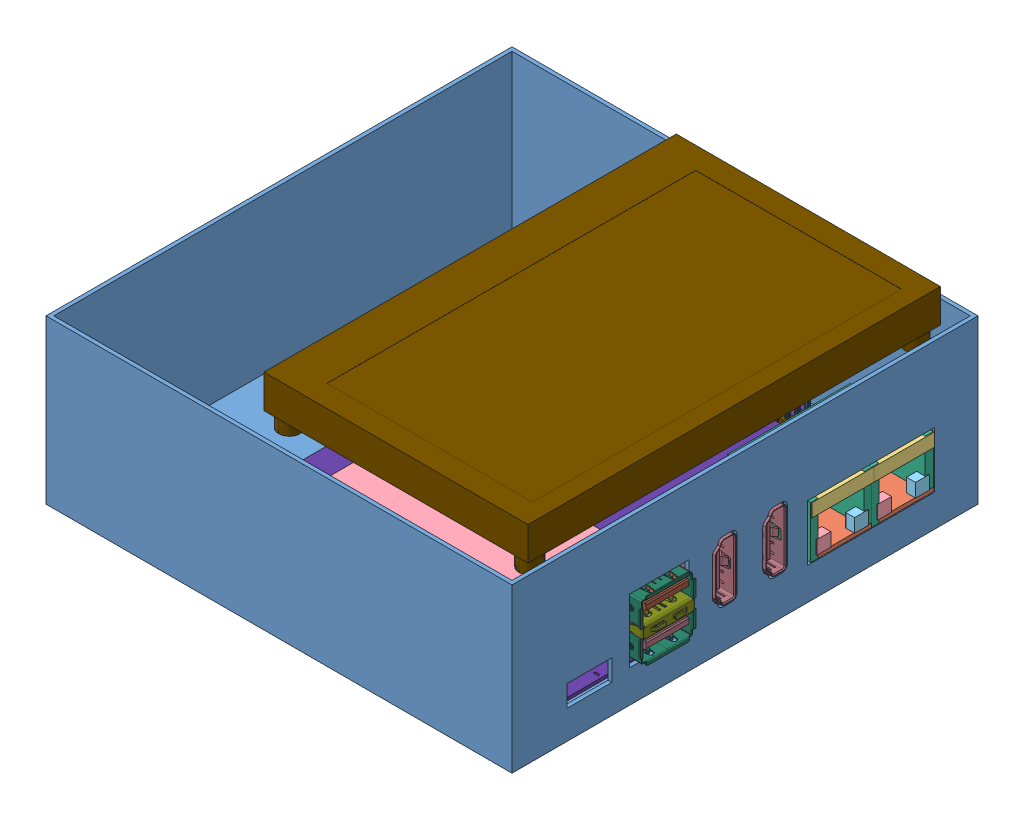
SolidWorks assembly bilbo-hub, configuration Default. Lengths in mm.
Overall size (123.13 50.39 120).
751 component instances, 90 part files, 5 mates.
Components (placement in the parent):
- box_lower-1: box_lower [Default] at origin size (120 42 120)
- CM4-DUAL-ETH-4G 5G-BASE-1: CM4-DUAL-ETH-4G 5G-BASE [Default] at (-27.9996 8.7984 -51.6437) x (1 0 0.000117) z (0 1 0) size (91.94 99.62 20.53)
  - CM4-DUAL-ETH-4G 5G-BASE.step-1: CM4-DUAL-ETH-4G 5G-BASE.step [Default] at origin size (91.94 99.62 20.53)
    - RJ1.step-1: RJ1.step [Default] at origin size (21.67 31.81 13.4)
      - 1103519632.step-1: 1103519632.step [Default] at (77.5484 -26.8671 0) size (21.44 15.98 1)
        - Extruded.step-1: Extruded.step [Default] at origin size (21.44 15.98 1)
      - 1103519760.step-1: 1103519760.step [Default] at (77.7643 -26.9433 10) size (21.46 15.98 3.4)
        - Extruded-0.step-1: Extruded-0.step [Default] at origin size (21.46 15.98 3.4)
      - 1314035072.step-1: 1314035072.step [Default] at (87.2916 -31.8201 1) size (2.34 3.63 3.5)
        - Extruded-1.step-1: Extruded-1.step [Default] at origin size (2.34 3.63 3.5)
      - 1314034944.step-1: 1314034944.step [Default] at (87.2408 -22.0157 1) size (2.34 3.63 3.5)
        - Extruded-2.step-1: Extruded-2.step [Default] at origin size (2.34 3.63 3.5)
      - 1314034816.step-1: 1314034816.step [Default] at (77.5611 -27.0322 0) size (21.46 15.95 13.4)
        - Extruded-3.step-1: Extruded-3.step [Default] at origin size (21.46 15.95 13.4)
      - 1314034816.step-2: 1314034816.step [Default] at (77.5611 -11.3472 0) size (21.46 15.95 13.4)
        - Extruded-3.step-1: Extruded-3.step [Default] at origin size (21.46 15.95 13.4)
      - 1314034944.step-2: 1314034944.step [Default] at (87.2408 -6.3307 1) size (2.34 3.63 3.5)
        - Extruded-2.step-1: Extruded-2.step [Default] at origin size (2.34 3.63 3.5)
      - 1314035072.step-2: 1314035072.step [Default] at (87.2916 -16.1351 1) size (2.34 3.63 3.5)
        - Extruded-1.step-1: Extruded-1.step [Default] at origin size (2.34 3.63 3.5)
      - 1103519760.step-2: 1103519760.step [Default] at (77.7643 -11.2583 10) size (21.46 15.98 3.4)
        - Extruded-0.step-1: Extruded-0.step [Default] at origin size (21.46 15.98 3.4)
      - 1103519632.step-2: 1103519632.step [Default] at (77.5484 -11.1821 0) size (21.44 15.98 1)
        - Extruded.step-1: Extruded.step [Default] at origin size (21.44 15.98 1)
    - R22.step-1: R22.step [Default] at origin size (1.65 0.85 0.46)
      - 575261968.step-1: 575261968.step [Default] at (69.9209 -91.4091 -1.2484) size (1.5 0.8 0.42)
        - Extruded-4.step-1: Extruded-4.step [Default] at origin size (1.5 0.8 0.42)
      - 575262096.step-1: 575262096.step [Default] at (70.6067 -91.4091 -1.2584) size (0.28 0.85 0.46)
        - Extruded-5.step-1: Extruded-5.step [Default] at origin size (0.28 0.85 0.46)
      - 575262096.step-2: 575262096.step [Default] at (69.2352 -91.4091 -1.2584) size (0.28 0.85 0.46)
        - Extruded-5.step-1: Extruded-5.step [Default] at origin size (0.28 0.85 0.46)
    - C2.step-1: C2.step [Default] at origin size (0.8 1.6 0.6)
      - CAPC1608(0603).step-1: CAPC1608(0603).step [Default] at (10.7694 -94.4916 -0.7984) x (0 -1 0) z (0 0 -1) size (1.6 0.8 0.6)
    - H7.step-1: H7.step [Default] at origin size (2.72 1.27 0.46)
      - 663598704.step-1: 663598704.step [Default] at (28.6963 -17.3457 -1.2484) size (2.29 1.12 0.42)
        - Extruded-6.step-1: Extruded-6.step [Default] at origin size (2.29 1.12 0.42)
      - 663598832.step-1: 663598832.step [Default] at (29.9768 -17.3457 -1.2584) size (0.28 1.27 0.46)
        - Extruded-7.step-1: Extruded-7.step [Default] at origin size (0.28 1.27 0.46)
      - 663598832.step-2: 663598832.step [Default] at (27.5279 -17.3457 -1.2584) size (0.28 1.27 0.46)
        - Extruded-7.step-1: Extruded-7.step [Default] at origin size (0.28 1.27 0.46)
    - R78.step-1: R78.step [Default] at origin size (1.65 0.85 0.46)
      - 575262096.step-1: 575262096.step [Default] at (63.7794 -84.0995 -1.2584) size (0.28 0.85 0.46)
        - Extruded-5.step-1: Extruded-5.step [Default] at origin size (0.28 0.85 0.46)
      - 575262096.step-2: 575262096.step [Default] at (62.4079 -84.0995 -1.2584) size (0.28 0.85 0.46)
        - Extruded-5.step-1: Extruded-5.step [Default] at origin size (0.28 0.85 0.46)
      - 575261968.step-1: 575261968.step [Default] at (63.0937 -84.0995 -1.2484) size (1.5 0.8 0.42)
        - Extruded-4.step-1: Extruded-4.step [Default] at origin size (1.5 0.8 0.42)
    - R39.step-1: R39.step [Default] at origin size (1.6 0.8 0.38)
      - RESC1608(0603).step-1: RESC1608(0603).step [Default] at (39.6845 -17.034 -0.7984) x (-1 0 0) z (0 -1 0) size (1.6 0.38 0.8)
    - R37.step-1: R37.step [Default] at origin size (1.6 0.8 0.38)
      - RESC1608(0603).step-1: RESC1608(0603).step [Default] at (39.6845 -15.3114 -0.7984) x (-1 0 0) z (0 -1 0) size (1.6 0.38 0.8)
    - R5.step-1: R5.step [Default] at origin size (1.6 0.8 0.38)
      - RESC1608(0603).step-1: RESC1608(0603).step [Default] at (39.8309 -21.4628 -0.7984) x (-1 0 0) z (0 -1 0) size (1.6 0.38 0.8)
    - R2.step-1: R2.step [Default] at origin size (1.6 0.8 0.38)
      - RESC1608(0603).step-1: RESC1608(0603).step [Default] at (39.8309 -24.5524 -0.7984) x (-1 0 0) z (0 -1 0) size (1.6 0.38 0.8)
    - R1.step-1: R1.step [Default] at origin size (1.6 0.8 0.38)
      - RESC1608(0603).step-1: RESC1608(0603).step [Default] at (39.8309 -23.0076 -0.7984) x (-1 0 0) z (0 -1 0) size (1.6 0.38 0.8)
    - H1.step-1: H1.step [Default] at origin size (1.6 0.8 0.38)
      - RESC1608(0603).step-1: RESC1608(0603).step [Default] at (30.6262 -13.3161 -0.7984) x (-1 0 0) z (0 -1 0) size (1.6 0.38 0.8)
    - H5.step-1: H5.step [Default] at origin size (1.6 0.8 0.38)
      - RESC1608(0603).step-1: RESC1608(0603).step [Default] at (30.6093 -24.1026 -0.7984) x (-1 0 0) z (0 -1 0) size (1.6 0.38 0.8)
    - H6.step-1: H6.step [Default] at origin size (1.6 0.8 0.38)
      - RESC1608(0603).step-1: RESC1608(0603).step [Default] at (30.6093 -21.9377 -0.7984) x (-1 0 0) z (0 -1 0) size (1.6 0.38 0.8)
    - R36.step-1: R36.step [Default] at origin size (1.6 0.8 0.38)
      - RESC1608(0603).step-1: RESC1608(0603).step [Default] at (39.6845 -13.5888 -0.7984) x (-1 0 0) z (0 -1 0) size (1.6 0.38 0.8)
    - HDMI1.step-1: HDMI1.step [Default] at origin size (23.1 7.88 20.15)
      - 72r3759_2007435-1.step-1: 72r3759_2007435-1.step [Default] at (88.2992 -43.8926 9) x (0 1 0) z (1 0 0) size (7.88 20.15 23.1)
    - U14.step-1: U14.step [Default] at origin size (1.7 1.81 0.55)
      - 1348844240.step-1: 1348844240.step [Default] at (15.1262 -53.2966 0.045) size (1.7 1.3 0.5)
        - Extruded-8.step-1: Extruded-8.step [Default] at origin size (1.7 1.3 0.5)
      - 764368800.step-1: 764368800.step [Default] at (15.6262 -52.5945 0) size (0.23 0.4 0.16)
        - Extruded-9.step-1: Extruded-9.step [Default] at origin size (0.23 0.4 0.16)
      - 764368800.step-2: 764368800.step [Default] at (15.1263 -52.5945 0) size (0.23 0.4 0.16)
        - Extruded-9.step-1: Extruded-9.step [Default] at origin size (0.23 0.4 0.16)
      - 764368800.step-3: 764368800.step [Default] at (14.6263 -52.5945 0) size (0.23 0.4 0.16)
        - Extruded-9.step-1: Extruded-9.step [Default] at origin size (0.23 0.4 0.16)
      - 764368800.step-4: 764368800.step [Default] at (14.6263 -53.9965 0) size (0.23 0.4 0.16)
        - Extruded-9.step-1: Extruded-9.step [Default] at origin size (0.23 0.4 0.16)
      - 764368800.step-5: 764368800.step [Default] at (15.1263 -53.9965 0) size (0.23 0.4 0.16)
        - Extruded-9.step-1: Extruded-9.step [Default] at origin size (0.23 0.4 0.16)
      - 764368800.step-6: 764368800.step [Default] at (15.6263 -53.9965 0) size (0.23 0.4 0.16)
        - Extruded-9.step-1: Extruded-9.step [Default] at origin size (0.23 0.4 0.16)
    - R73.step-1: R73.step [Default] at origin size (0.8 1.6 0.38)
      - RESC1608(0603).step-1: RESC1608(0603).step [Default] at (13.494 -56.6964 0) x (0 1 0) z (1 0 0) size (1.6 0.38 0.8)
    - R72.step-1: R72.step [Default] at origin size (0.8 1.6 0.38)
      - RESC1608(0603).step-1: RESC1608(0603).step [Default] at (15.2725 -56.7662 0) x (0 -1 0) z (-1 0 0) size (1.6 0.38 0.8)
    - R71.step-1: R71.step [Default] at origin size (0.8 1.6 0.38)
      - RESC1608(0603).step-1: RESC1608(0603).step [Default] at (11.7419 -56.7662 0) x (0 -1 0) z (-1 0 0) size (1.6 0.38 0.8)
    - R70.step-1: R70.step [Default] at origin size (0.8 1.6 0.38)
      - RESC1608(0603).step-1: RESC1608(0603).step [Default] at (18.8031 -56.7662 0) x (0 -1 0) z (-1 0 0) size (1.6 0.38 0.8)
    - R69.step-1: R69.step [Default] at origin size (1.6 0.8 0.38)
      - RESC1608(0603).step-1: RESC1608(0603).step [Default] at (12.4687 -54.179 0) x (1 0 0) z (0 -1 0) size (1.6 0.38 0.8)
    - L7.step-1: L7.step [Default] at origin size (6.5 7.2 2.9)
      - 1127965152.step-1: 1127965152.step [Default] at (17.9746 -48.1322 -3.7984) size (6.5 7.2 2.9)
        - Extruded-10.step-1: Extruded-10.step [Default] at origin size (6.5 7.2 2.9)
    - KEY1.step-1: KEY1.step [Default] at origin size (3.6 9 8.45)
      - User_Library-MMP221.step-1: User_Library-MMP221.step [Default] at (3.4634 -45.8936 0) x (0 1 0) z (1 0 0) size (9 8.45 3.6)
        - User_Library-MMP221_MMP221.step-1: User_Library-MMP221_MMP221.step [Default] at (0 3.3 0) x (-1 0 0) z (0 0 1) size (8.9 3.3 3.6)
        - User_Library-MMP221_MMP221_SM.step-1: User_Library-MMP221_MMP221_SM.step [Default] at (0 3.3 0) x (-1 0 0) z (0 0 -1) size (9 2.1 3.6)
        - User_Library-MMP221_MMP221_PP.step-1: User_Library-MMP221_MMP221_PP.step [Default] at (1 1.2 0) x (-1 0 0) z (0 0 -1) size (6 4.3 2.6)
        - User_Library-MMP221_MMP221_PIN.step-1: User_Library-MMP221_MMP221_PIN.step [Default] at (0 1.05 0) size (0.6 4 3.2)
        - User_Library-MMP221_MMP221_PIN.step-2: User_Library-MMP221_MMP221_PIN.step [Default] at (2.5 1.05 0) size (0.6 4 3.2)
        - User_Library-MMP221_MMP221_PIN.step-3: User_Library-MMP221_MMP221_PIN.step [Default] at (-2.5 1.05 0) size (0.6 4 3.2)
    - C102.step-1: C102.step [Default] at origin size (1.6 0.8 0.6)
      - CAPC1608(0603).step-1: CAPC1608(0603).step [Default] at (19.7102 -43.0166 -0.7984) x (-1 0 0) z (0 0 -1) size (1.6 0.8 0.6)
    - C101.step-1: C101.step [Default] at origin size (1.6 0.8 0.6)
      - CAPC1608(0603).step-1: CAPC1608(0603).step [Default] at (16.3525 -43.0371 -0.7984) x (1 0 0) z (0 0 -1) size (1.6 0.8 0.6)
    - C100.step-1: C100.step [Default] at origin size (0.8 1.6 0.6)
      - CAPC1608(0603).step-1: CAPC1608(0603).step [Default] at (17.0311 -56.7181 0) x (0 1 0) z (0 0 1) size (1.6 0.8 0.6)
    - C99.step-1: C99.step [Default] at origin size (1.6 0.8 0.6)
      - CAPC1608(0603).step-1: CAPC1608(0603).step [Default] at (18.1108 -54.2618 0) x (1 0 0) z (0 0 1) size (1.6 0.8 0.6)
    - C98.step-1: C98.step [Default] at origin size (1.6 0.8 0.6)
      - CAPC1608(0603).step-1: CAPC1608(0603).step [Default] at (18.0852 -52.5347 0) x (-1 0 0) z (0 0 1) size (1.6 0.8 0.6)
    - C97.step-1: C97.step [Default] at origin size (1.6 0.8 0.6)
      - CAPC1608(0603).step-1: CAPC1608(0603).step [Default] at (12.3956 -52.4839 0) x (-1 0 0) z (0 0 1) size (1.6 0.8 0.6)
    - TVS1.step-1: TVS1.step [Default] at origin size (2.26 2 1.05)
      - User_Library-SOT-363.step-1: User_Library-SOT-363.step [Default] at (18.2037 -82.092 0) x (0 -1 0) z (0 0 1) size (2 2.26 1.05)
    - SIMCOM1.step-1: SIMCOM1.step [Default] at origin size (56.01 29.97 4.02)
      - 663597680.step-1: 663597680.step [Default] at (34.593 -73.1988 2) size (48.01 29.97 1.5)
        - Extruded-11.step-1: Extruded-11.step [Default] at origin size (48.01 29.97 1.5)
      - 89w2147_2199119-3.step-1: 89w2147_2199119-3.step [Default] at (58.246 -73.1627 1.8) x (0 -1 0) z (-1 0 0) size (21.9 3.7 8.7)
    - R65.step-1: R65.step [Default] at origin size (1.6 0.8 0.38)
      - RESC1608(0603).step-1: RESC1608(0603).step [Default] at (18.2734 -80.3285 0) x (1 0 0) z (0 -1 0) size (1.6 0.38 0.8)
    - R63.step-1: R63.step [Default] at origin size (1.6 0.8 0.38)
      - RESC1608(0603).step-1: RESC1608(0603).step [Default] at (18.2734 -83.8424 0) x (1 0 0) z (0 -1 0) size (1.6 0.38 0.8)
    - R62.step-1: R62.step [Default] at origin size (1.6 0.8 0.38)
      - RESC1608(0603).step-1: RESC1608(0603).step [Default] at (18.2036 -85.6126 0) x (-1 0 0) z (0 1 0) size (1.6 0.38 0.8)
    - R61.step-1: R61.step [Default] at origin size (1.6 0.8 0.38)
      - RESC1608(0603).step-1: RESC1608(0603).step [Default] at (52.8513 -64.7592 0) x (1 0 0) z (0 -1 0) size (1.6 0.38 0.8)
    - R60.step-1: R60.step [Default] at origin size (1.6 0.8 0.38)
      - RESC1608(0603).step-1: RESC1608(0603).step [Default] at (10.7955 -82.0987 0) x (-1 0 0) z (0 1 0) size (1.6 0.38 0.8)
    - R59.step-1: R59.step [Default] at origin size (1.6 0.8 0.38)
      - RESC1608(0603).step-1: RESC1608(0603).step [Default] at (10.7955 -80.3417 0) x (-1 0 0) z (0 1 0) size (1.6 0.38 0.8)
    - R58.step-1: R58.step [Default] at origin size (1.6 0.8 0.38)
      - RESC1608(0603).step-1: RESC1608(0603).step [Default] at (52.7894 -81.5725 0) x (-1 0 0) z (0 1 0) size (1.6 0.38 0.8)
    - R54.step-1: R54.step [Default] at origin size (1.6 0.8 0.38)
      - RESC1608(0603).step-1: RESC1608(0603).step [Default] at (52.8617 -73.2495 0) x (1 0 0) z (0 -1 0) size (1.6 0.38 0.8)
    - R53.step-1: R53.step [Default] at origin size (1.6 0.8 0.38)
      - RESC1608(0603).step-1: RESC1608(0603).step [Default] at (52.8592 -79.9158 0) x (1 0 0) z (0 -1 0) size (1.6 0.38 0.8)
    - R52.step-1: R52.step [Default] at origin size (1.6 0.8 0.38)
      - RESC1608(0603).step-1: RESC1608(0603).step [Default] at (52.7894 -74.8236 0) x (-1 0 0) z (0 1 0) size (1.6 0.38 0.8)
    - R51.step-1: R51.step [Default] at origin size (1.6 0.8 0.38)
      - RESC1608(0603).step-1: RESC1608(0603).step [Default] at (52.7894 -71.7017 0) x (-1 0 0) z (0 1 0) size (1.6 0.38 0.8)
    - R50.step-1: R50.step [Default] at origin size (1.6 0.8 0.38)
      - RESC1608(0603).step-1: RESC1608(0603).step [Default] at (52.7894 -70.1694 0) x (-1 0 0) z (0 1 0) size (1.6 0.38 0.8)
    - Q7.step-1: Q7.step [Default] at origin size (2.64 3 1.08)
      - ALSRobot-SOT23.step-1: ALSRobot-SOT23.step [Default] at (52.8095 -67.5135 0) x (0 -1 0) z (0 0 1) size (3 2.64 1.08)
    - Q6.step-1: Q6.step [Default] at origin size (2.64 3 1.08)
      - ALSRobot-SOT23.step-1: ALSRobot-SOT23.step [Default] at (52.8174 -77.2017 0) x (0 -1 0) z (0 0 1) size (3 2.64 1.08)
    - L4.step-1: L4.step [Default] at origin size (9.95 4.45 11.5)
      - 1015527712.step-1: 1015527712.step [Default] at (0.9405 -66.9019 3) x (0 -1 0) z (0 0 1) size (3.5 3.5 3.5)
        - Sphere.step-1: Sphere.step [Default] at origin size (3.5 3.5 3.5)
      - 1103520528.step-1: 1103520528.step [Default] at (4.6411 -66.9011 0.254) size (9 4.45 9.75)
        - Extruded-12.step-1: Extruded-12.step [Default] at origin size (9 4.45 9.75)
      - 1015527832.step-1: 1015527832.step [Default] at (0.9405 -66.9019 8) x (0 -1 0) z (0 0 1) size (3.5 3.5 3.5)
        - Sphere-13.step-1: Sphere-13.step [Default] at origin size (3.5 3.5 3.5)
      - 1015527952.step-1: 1015527952.step [Default] at (7.7605 -65.6318 -1.5) x (0 1 0) z (0 0 1) size (0.76 0.76 5)
        - Cylinder.step-1: Cylinder.step [Default] at origin size (0.76 0.76 5)
      - 1015527952.step-2: 1015527952.step [Default] at (5.2205 -65.6318 -1.5) x (0 1 0) z (0 0 1) size (0.76 0.76 5)
        - Cylinder.step-1: Cylinder.step [Default] at origin size (0.76 0.76 5)
      - 1015527952.step-3: 1015527952.step [Default] at (5.2205 -68.1718 -1.5) x (0 1 0) z (0 0 1) size (0.76 0.76 5)
        - Cylinder.step-1: Cylinder.step [Default] at origin size (0.76 0.76 5)
      - 1015527952.step-4: 1015527952.step [Default] at (7.7605 -68.1718 -1.5) x (0 1 0) z (0 0 1) size (0.76 0.76 5)
        - Cylinder.step-1: Cylinder.step [Default] at origin size (0.76 0.76 5)
    - C94.step-1: C94.step [Default] at origin size (1.6 0.8 0.6)
      - CAPC1608(0603).step-1: CAPC1608(0603).step [Default] at (14.7077 -80.335 0) x (1 0 0) z (0 0 1) size (1.6 0.8 0.6)
    - C92.step-1: C92.step [Default] at origin size (1.6 0.8 0.6)
      - CAPC1608(0603).step-1: CAPC1608(0603).step [Default] at (14.7077 -85.6059 0) x (1 0 0) z (0 0 1) size (1.6 0.8 0.6)
    - C91.step-1: C91.step [Default] at origin size (1.6 0.8 0.6)
      - CAPC1608(0603).step-1: CAPC1608(0603).step [Default] at (14.7077 -82.092 0) x (1 0 0) z (0 0 1) size (1.6 0.8 0.6)
    - C90.step-1: C90.step [Default] at origin size (0.8 1.6 0.6)
      - CAPC1608(0603).step-1: CAPC1608(0603).step [Default] at (45.5624 -61.984 0) x (0 1 0) z (0 0 1) size (1.6 0.8 0.6)
    - C89.step-1: C89.step [Default] at origin size (0.8 1.6 0.6)
      - CAPC1608(0603).step-1: CAPC1608(0603).step [Default] at (44.0637 -61.984 0) x (0 1 0) z (0 0 1) size (1.6 0.8 0.6)
    - C88.step-1: C88.step [Default] at origin size (0.8 1.6 0.6)
      - CAPC1608(0603).step-1: CAPC1608(0603).step [Default] at (77.2669 -88.5749 -0.7984) x (0 1 0) z (0 0 -1) size (1.6 0.8 0.6)
    - J1.step-1: J1.step [Default] at origin size (20.5 15.59 19.61)
      - 44000.step-1: 44000.step [Default] at (72.6815 -73.7566 7.8016) x (-1 0 0) z (0 0 -1) size (20.5 15.59 19.61)
        - SOLID.step-1: SOLID.step [Default] at origin size (19.25 11.1 2.6)
        - SOLID-14.step-1: SOLID-14.step [Default] at origin size (19.3 13.3 15.01)
        - SOLID-15.step-1: SOLID-15.step [Default] at origin size (19.25 11.1 2.6)
        - SOLID-16.step-1: SOLID-16.step [Default] at origin size (5.49 11.5 14.69)
        - SOLID-17.step-1: SOLID-17.step [Default] at origin size (18.21 1.45 17.25)
        - SOLID-18.step-1: SOLID-18.step [Default] at origin size (18.21 1.45 17.25)
        - SOLID-19.step-1: SOLID-19.step [Default] at origin size (18.21 1.45 17.25)
        - SOLID-20.step-1: SOLID-20.step [Default] at origin size (18.21 1.45 17.25)
        - SOLID-21.step-1: SOLID-21.step [Default] at origin size (18.21 1.45 17.25)
        - SOLID-22.step-1: SOLID-22.step [Default] at origin size (12.91 1 15.85)
        - SOLID-23.step-1: SOLID-23.step [Default] at origin size (12.91 1 15.85)
        - SOLID-24.step-1: SOLID-24.step [Default] at origin size (12.91 1 15.81)
        - SOLID-25.step-1: SOLID-25.step [Default] at origin size (12.91 1 15.81)
        - SOLID-26.step-1: SOLID-26.step [Default] at origin size (15.01 1.45 8.75)
        - SOLID-27.step-1: SOLID-27.step [Default] at origin size (15.01 1.45 8.75)
        - SOLID-28.step-1: SOLID-28.step [Default] at origin size (15.01 1.45 8.75)
        - SOLID-29.step-1: SOLID-29.step [Default] at origin size (15.01 1.45 8.75)
        - SOLID-30.step-1: SOLID-30.step [Default] at origin size (15.01 1.45 8.75)
        - SOLID-31.step-1: SOLID-31.step [Default] at origin size (10.42 1 7.35)
        - SOLID-32.step-1: SOLID-32.step [Default] at origin size (10.42 1 7.35)
        - SOLID-33.step-1: SOLID-33.step [Default] at origin size (10.42 1 7.35)
        - SOLID-34.step-1: SOLID-34.step [Default] at origin size (10.42 1 7.35)
        - SOLID-35.step-1: SOLID-35.step [Default] at origin size (19.7 15.59 19.61)
        - SOLID-36.step-1: SOLID-36.step [Default] at origin size (16.1 13.62 4.38)
    - PI1.step-1: PI1.step [Default] at origin size (50.58 4.88 11.2)
      - 1466328752.step-1: 1466328752.step [Default] at (9.6693 -4.3696 0) size (4.86 2.63 1.1)
        - Extruded-37.step-1: Extruded-37.step [Default] at origin size (4.86 2.63 1.1)
      - 1503596240.step-1: 1503596240.step [Default] at (9.6693 -6.7686 0) size (4.86 2.33 1.1)
        - Extruded-38.step-1: Extruded-38.step [Default] at origin size (4.86 2.33 1.1)
      - 1503596240.step-2: 1503596240.step [Default] at (14.7493 -6.7686 0) size (4.86 2.33 1.1)
        - Extruded-38.step-1: Extruded-38.step [Default] at origin size (4.86 2.33 1.1)
      - 1466328752.step-2: 1466328752.step [Default] at (14.7493 -4.3696 0) size (4.86 2.63 1.1)
        - Extruded-37.step-1: Extruded-37.step [Default] at origin size (4.86 2.63 1.1)
      - 1503596240.step-3: 1503596240.step [Default] at (19.8293 -6.7686 0) size (4.86 2.33 1.1)
        - Extruded-38.step-1: Extruded-38.step [Default] at origin size (4.86 2.33 1.1)
      - 1466328752.step-3: 1466328752.step [Default] at (19.8293 -4.3696 0) size (4.86 2.63 1.1)
        - Extruded-37.step-1: Extruded-37.step [Default] at origin size (4.86 2.63 1.1)
      - 1503596240.step-4: 1503596240.step [Default] at (24.9093 -6.7686 0) size (4.86 2.33 1.1)
        - Extruded-38.step-1: Extruded-38.step [Default] at origin size (4.86 2.33 1.1)
      - 1466328752.step-4: 1466328752.step [Default] at (24.9093 -4.3696 0) size (4.86 2.63 1.1)
        - Extruded-37.step-1: Extruded-37.step [Default] at origin size (4.86 2.63 1.1)
      - 1503596240.step-5: 1503596240.step [Default] at (29.9893 -6.7686 0) size (4.86 2.33 1.1)
        - Extruded-38.step-1: Extruded-38.step [Default] at origin size (4.86 2.33 1.1)
      - 1466328752.step-5: 1466328752.step [Default] at (29.9893 -4.3696 0) size (4.86 2.63 1.1)
        - Extruded-37.step-1: Extruded-37.step [Default] at origin size (4.86 2.63 1.1)
      - 1503596240.step-6: 1503596240.step [Default] at (35.0693 -6.7686 0) size (4.86 2.33 1.1)
        - Extruded-38.step-1: Extruded-38.step [Default] at origin size (4.86 2.33 1.1)
      - 1466328752.step-6: 1466328752.step [Default] at (35.0693 -4.3696 0) size (4.86 2.63 1.1)
        - Extruded-37.step-1: Extruded-37.step [Default] at origin size (4.86 2.63 1.1)
      - 1503596240.step-7: 1503596240.step [Default] at (40.1493 -6.7686 0) size (4.86 2.33 1.1)
        - Extruded-38.step-1: Extruded-38.step [Default] at origin size (4.86 2.33 1.1)
      - 1466328752.step-7: 1466328752.step [Default] at (40.1493 -4.3696 0) size (4.86 2.63 1.1)
        - Extruded-37.step-1: Extruded-37.step [Default] at origin size (4.86 2.63 1.1)
      - 1503596240.step-8: 1503596240.step [Default] at (45.2293 -6.7686 0) size (4.86 2.33 1.1)
        - Extruded-38.step-1: Extruded-38.step [Default] at origin size (4.86 2.33 1.1)
      - 1466328752.step-8: 1466328752.step [Default] at (45.2293 -4.3696 0) size (4.86 2.63 1.1)
        - Extruded-37.step-1: Extruded-37.step [Default] at origin size (4.86 2.63 1.1)
      - 1503596240.step-9: 1503596240.step [Default] at (50.3093 -6.7686 0) size (4.86 2.33 1.1)
        - Extruded-38.step-1: Extruded-38.step [Default] at origin size (4.86 2.33 1.1)
      - 1466328752.step-9: 1466328752.step [Default] at (50.3093 -4.3696 0) size (4.86 2.63 1.1)
        - Extruded-37.step-1: Extruded-37.step [Default] at origin size (4.86 2.63 1.1)
      - 1503596240.step-10: 1503596240.step [Default] at (55.3893 -6.7686 0) size (4.86 2.33 1.1)
        - Extruded-38.step-1: Extruded-38.step [Default] at origin size (4.86 2.33 1.1)
      - 1466328752.step-10: 1466328752.step [Default] at (55.3893 -4.3696 0) size (4.86 2.63 1.1)
        - Extruded-37.step-1: Extruded-37.step [Default] at origin size (4.86 2.63 1.1)
      - 1466328880.step-1: 1466328880.step [Default] at (8.3884 -6.781 -2.2) size (1.11 1.11 11.2)
        - Extruded-39.step-1: Extruded-39.step [Default] at origin size (1.11 1.11 11.2)
      - 1466328880.step-2: 1466328880.step [Default] at (8.3884 -4.241 -2.2) size (1.11 1.11 11.2)
        - Extruded-39.step-1: Extruded-39.step [Default] at origin size (1.11 1.11 11.2)
      - 1466328880.step-3: 1466328880.step [Default] at (10.9285 -6.781 -2.2) size (1.11 1.11 11.2)
        - Extruded-39.step-1: Extruded-39.step [Default] at origin size (1.11 1.11 11.2)
      - 1466328880.step-4: 1466328880.step [Default] at (10.9285 -4.241 -2.2) size (1.11 1.11 11.2)
        - Extruded-39.step-1: Extruded-39.step [Default] at origin size (1.11 1.11 11.2)
      - 1466328880.step-5: 1466328880.step [Default] at (13.4685 -6.781 -2.2) size (1.11 1.11 11.2)
        - Extruded-39.step-1: Extruded-39.step [Default] at origin size (1.11 1.11 11.2)
      - 1466328880.step-6: 1466328880.step [Default] at (13.4685 -4.241 -2.2) size (1.11 1.11 11.2)
        - Extruded-39.step-1: Extruded-39.step [Default] at origin size (1.11 1.11 11.2)
      - 1466328880.step-7: 1466328880.step [Default] at (16.0085 -6.781 -2.2) size (1.11 1.11 11.2)
        - Extruded-39.step-1: Extruded-39.step [Default] at origin size (1.11 1.11 11.2)
      - 1466328880.step-8: 1466328880.step [Default] at (16.0085 -4.241 -2.2) size (1.11 1.11 11.2)
        - Extruded-39.step-1: Extruded-39.step [Default] at origin size (1.11 1.11 11.2)
      - 1466328880.step-9: 1466328880.step [Default] at (18.5484 -6.781 -2.2) size (1.11 1.11 11.2)
        - Extruded-39.step-1: Extruded-39.step [Default] at origin size (1.11 1.11 11.2)
      - 1466328880.step-10: 1466328880.step [Default] at (18.5484 -4.241 -2.2) size (1.11 1.11 11.2)
        - Extruded-39.step-1: Extruded-39.step [Default] at origin size (1.11 1.11 11.2)
      - 1466328880.step-11: 1466328880.step [Default] at (21.0885 -6.781 -2.2) size (1.11 1.11 11.2)
        - Extruded-39.step-1: Extruded-39.step [Default] at origin size (1.11 1.11 11.2)
      - 1466328880.step-12: 1466328880.step [Default] at (21.0885 -4.241 -2.2) size (1.11 1.11 11.2)
        - Extruded-39.step-1: Extruded-39.step [Default] at origin size (1.11 1.11 11.2)
      - 1466328880.step-13: 1466328880.step [Default] at (23.6285 -6.781 -2.2) size (1.11 1.11 11.2)
        - Extruded-39.step-1: Extruded-39.step [Default] at origin size (1.11 1.11 11.2)
      - 1466328880.step-14: 1466328880.step [Default] at (23.6285 -4.241 -2.2) size (1.11 1.11 11.2)
        - Extruded-39.step-1: Extruded-39.step [Default] at origin size (1.11 1.11 11.2)
      - 1466328880.step-15: 1466328880.step [Default] at (26.1685 -6.781 -2.2) size (1.11 1.11 11.2)
        - Extruded-39.step-1: Extruded-39.step [Default] at origin size (1.11 1.11 11.2)
      - 1466328880.step-16: 1466328880.step [Default] at (26.1685 -4.241 -2.2) size (1.11 1.11 11.2)
        - Extruded-39.step-1: Extruded-39.step [Default] at origin size (1.11 1.11 11.2)
      - 1466328880.step-17: 1466328880.step [Default] at (28.7084 -6.781 -2.2) size (1.11 1.11 11.2)
        - Extruded-39.step-1: Extruded-39.step [Default] at origin size (1.11 1.11 11.2)
      - 1466328880.step-18: 1466328880.step [Default] at (28.7084 -4.241 -2.2) size (1.11 1.11 11.2)
        - Extruded-39.step-1: Extruded-39.step [Default] at origin size (1.11 1.11 11.2)
      - 1466328880.step-19: 1466328880.step [Default] at (31.2485 -6.781 -2.2) size (1.11 1.11 11.2)
        - Extruded-39.step-1: Extruded-39.step [Default] at origin size (1.11 1.11 11.2)
      - 1466328880.step-20: 1466328880.step [Default] at (31.2485 -4.241 -2.2) size (1.11 1.11 11.2)
        - Extruded-39.step-1: Extruded-39.step [Default] at origin size (1.11 1.11 11.2)
      - 1466328880.step-21: 1466328880.step [Default] at (33.7885 -6.781 -2.2) size (1.11 1.11 11.2)
        - Extruded-39.step-1: Extruded-39.step [Default] at origin size (1.11 1.11 11.2)
      - 1466328880.step-22: 1466328880.step [Default] at (33.7885 -4.241 -2.2) size (1.11 1.11 11.2)
        - Extruded-39.step-1: Extruded-39.step [Default] at origin size (1.11 1.11 11.2)
      - 1466328880.step-23: 1466328880.step [Default] at (36.3284 -6.781 -2.2) size (1.11 1.11 11.2)
        - Extruded-39.step-1: Extruded-39.step [Default] at origin size (1.11 1.11 11.2)
      - 1466328880.step-24: 1466328880.step [Default] at (36.3284 -4.241 -2.2) size (1.11 1.11 11.2)
        - Extruded-39.step-1: Extruded-39.step [Default] at origin size (1.11 1.11 11.2)
      - 1466328880.step-25: 1466328880.step [Default] at (38.8685 -6.781 -2.2) size (1.11 1.11 11.2)
        - Extruded-39.step-1: Extruded-39.step [Default] at origin size (1.11 1.11 11.2)
      - 1466328880.step-26: 1466328880.step [Default] at (38.8685 -4.241 -2.2) size (1.11 1.11 11.2)
        - Extruded-39.step-1: Extruded-39.step [Default] at origin size (1.11 1.11 11.2)
      - 1466328880.step-27: 1466328880.step [Default] at (41.4085 -6.781 -2.2) size (1.11 1.11 11.2)
        - Extruded-39.step-1: Extruded-39.step [Default] at origin size (1.11 1.11 11.2)
      - 1466328880.step-28: 1466328880.step [Default] at (41.4085 -4.241 -2.2) size (1.11 1.11 11.2)
        - Extruded-39.step-1: Extruded-39.step [Default] at origin size (1.11 1.11 11.2)
      - 1466328880.step-29: 1466328880.step [Default] at (43.9485 -6.781 -2.2) size (1.11 1.11 11.2)
        - Extruded-39.step-1: Extruded-39.step [Default] at origin size (1.11 1.11 11.2)
      - 1466328880.step-30: 1466328880.step [Default] at (43.9485 -4.241 -2.2) size (1.11 1.11 11.2)
        - Extruded-39.step-1: Extruded-39.step [Default] at origin size (1.11 1.11 11.2)
      - 1466328880.step-31: 1466328880.step [Default] at (46.4884 -6.781 -2.2) size (1.11 1.11 11.2)
        - Extruded-39.step-1: Extruded-39.step [Default] at origin size (1.11 1.11 11.2)
      - 1466328880.step-32: 1466328880.step [Default] at (46.4884 -4.241 -2.2) size (1.11 1.11 11.2)
        - Extruded-39.step-1: Extruded-39.step [Default] at origin size (1.11 1.11 11.2)
      - 1466328880.step-33: 1466328880.step [Default] at (49.0285 -6.781 -2.2) size (1.11 1.11 11.2)
        - Extruded-39.step-1: Extruded-39.step [Default] at origin size (1.11 1.11 11.2)
      - 1466328880.step-34: 1466328880.step [Default] at (49.0285 -4.241 -2.2) size (1.11 1.11 11.2)
        - Extruded-39.step-1: Extruded-39.step [Default] at origin size (1.11 1.11 11.2)
      - 1466328880.step-35: 1466328880.step [Default] at (51.5685 -6.781 -2.2) size (1.11 1.11 11.2)
        - Extruded-39.step-1: Extruded-39.step [Default] at origin size (1.11 1.11 11.2)
      - 1466328880.step-36: 1466328880.step [Default] at (51.5685 -4.241 -2.2) size (1.11 1.11 11.2)
        - Extruded-39.step-1: Extruded-39.step [Default] at origin size (1.11 1.11 11.2)
      - 1466328880.step-37: 1466328880.step [Default] at (54.1084 -6.781 -2.2) size (1.11 1.11 11.2)
        - Extruded-39.step-1: Extruded-39.step [Default] at origin size (1.11 1.11 11.2)
      - 1466328880.step-38: 1466328880.step [Default] at (54.1084 -4.241 -2.2) size (1.11 1.11 11.2)
        - Extruded-39.step-1: Extruded-39.step [Default] at origin size (1.11 1.11 11.2)
      - 1466328880.step-39: 1466328880.step [Default] at (56.6485 -6.781 -2.2) size (1.11 1.11 11.2)
        - Extruded-39.step-1: Extruded-39.step [Default] at origin size (1.11 1.11 11.2)
      - 1466328880.step-40: 1466328880.step [Default] at (56.6485 -4.241 -2.2) size (1.11 1.11 11.2)
        - Extruded-39.step-1: Extruded-39.step [Default] at origin size (1.11 1.11 11.2)
    - R19.step-1: R19.step [Default] at origin size (0.8 1.6 0.38)
      - RESC1608(0603).step-1: RESC1608(0603).step [Default] at (55.2872 -41.4682 -0.7984) x (0 -1 0) z (1 0 0) size (1.6 0.38 0.8)
    - R7.step-1: R7.step [Default] at origin size (0.8 1.6 0.38)
      - RESC1608(0603).step-1: RESC1608(0603).step [Default] at (56.8229 -41.4682 -0.7984) x (0 -1 0) z (1 0 0) size (1.6 0.38 0.8)
    - C85.step-1: C85.step [Default] at origin size (1.6 0.8 0.6)
      - CAPC1608(0603).step-1: CAPC1608(0603).step [Default] at (11.4504 -68.9687 -0.7984) x (1 0 0) z (0 0 -1) size (1.6 0.8 0.6)
    - R42.step-1: R42.step [Default] at origin size (1.6 0.8 0.38)
      - RESC1608(0603).step-1: RESC1608(0603).step [Default] at (20.7078 -68.9867 -0.7984) x (-1 0 0) z (0 -1 0) size (1.6 0.38 0.8)
    - R41.step-1: R41.step [Default] at origin size (1.6 0.8 0.38)
      - RESC1608(0603).step-1: RESC1608(0603).step [Default] at (16.0306 -68.9783 -0.7984) x (-1 0 0) z (0 -1 0) size (1.6 0.38 0.8)
    - L2.step-1: L2.step [Default] at origin size (4.4 4 1.97)
      - 764368672.step-1: 764368672.step [Default] at (12.0725 -60.2189 -2.7984) size (4.4 4 1.97)
        - Extruded-40.step-1: Extruded-40.step [Default] at origin size (4.4 4 1.97)
    - IN1.step-1: IN1.step [Default] at origin size (5.08 2.54 2.29)
      - 880594368.step-1: 880594368.step [Default] at (13.1901 -55.881 -3.0844) size (5.08 2.54 2.29)
        - Extruded-41.step-1: Extruded-41.step [Default] at origin size (5.08 2.54 2.29)
    - C86.step-1: C86.step [Default] at origin size (1.6 0.8 0.6)
      - CAPC1608(0603).step-1: CAPC1608(0603).step [Default] at (20.7558 -65.5584 -0.7984) x (1 0 0) z (0 0 -1) size (1.6 0.8 0.6)
    - C81.step-1: C81.step [Default] at origin size (3.2 1.6 1.1)
      - INDC3216(1206).step-1: INDC3216(1206).step [Default] at (19.7687 -55.8531 -0.7984) x (1 0 0) z (0 1 0) size (3.2 1.1 1.6)
    - Y1.step-1: Y1.step [Default] at origin size (3.95 3.1 1)
      - 1081399232.step-1: 1081399232.step [Default] at (55.2454 -27.8136 -1.7984) size (3.95 3.1 1)
        - Extruded-42.step-1: Extruded-42.step [Default] at origin size (3.95 3.1 1)
    - U6.step-1: U6.step [Default] at origin size (5 5 0.83)
      - 575262992.step-1: 575262992.step [Default] at (57.6658 -34.957 -1.6484) size (5 5 0.83)
        - Extruded-43.step-1: Extruded-43.step [Default] at origin size (5 5 0.83)
    - Y3.step-1: Y3.step [Default] at origin size (3.95 3.1 1)
      - 1081399232.step-1: 1081399232.step [Default] at (43.0933 -80.7653 0) size (3.95 3.1 1)
        - Extruded-42.step-1: Extruded-42.step [Default] at origin size (3.95 3.1 1)
    - U7.step-1: U7.step [Default] at origin size (8.1 8.1 0.83)
      - 880596288.step-1: 880596288.step [Default] at (39.1687 -70.7339 0.02) size (8.1 8.1 0.83)
        - Extruded-44.step-1: Extruded-44.step [Default] at origin size (8.1 8.1 0.83)
    - R31.step-1: R31.step [Default] at origin size (1.6 0.8 0.38)
      - RESC1608(0603).step-1: RESC1608(0603).step [Default] at (29.9452 -67.4397 0) x (1 0 0) z (0 -1 0) size (1.6 0.38 0.8)
    - R29.step-1: R29.step [Default] at origin size (1.6 0.8 0.38)
      - RESC1608(0603).step-1: RESC1608(0603).step [Default] at (51.4841 -34.1268 -0.7984) x (-1 0 0) z (0 -1 0) size (1.6 0.38 0.8)
    - R28.step-1: R28.step [Default] at origin size (0.8 1.6 0.38)
      - RESC1608(0603).step-1: RESC1608(0603).step [Default] at (47.9001 -80.8002 0) x (0 -1 0) z (-1 0 0) size (1.6 0.38 0.8)
    - R27.step-1: R27.step [Default] at origin size (0.8 1.6 0.38)
      - RESC1608(0603).step-1: RESC1608(0603).step [Default] at (49.5511 -80.9018 0) x (0 -1 0) z (-1 0 0) size (1.6 0.38 0.8)
    - R26.step-1: R26.step [Default] at origin size (1.6 0.8 0.38)
      - RESC1608(0603).step-1: RESC1608(0603).step [Default] at (29.8754 -64.5414 0) x (-1 0 0) z (0 1 0) size (1.6 0.38 0.8)
    - R25.step-1: R25.step [Default] at origin size (0.8 1.6 0.38)
      - RESC1608(0603).step-1: RESC1608(0603).step [Default] at (30.9892 -80.8002 0) x (0 -1 0) z (-1 0 0) size (1.6 0.38 0.8)
    - R24.step-1: R24.step [Default] at origin size (0.8 1.6 0.38)
      - RESC1608(0603).step-1: RESC1608(0603).step [Default] at (32.7864 -80.8002 0) x (0 -1 0) z (-1 0 0) size (1.6 0.38 0.8)
    - R23.step-1: R23.step [Default] at origin size (0.8 1.6 0.38)
      - RESC1608(0603).step-1: RESC1608(0603).step [Default] at (34.5836 -80.8002 0) x (0 -1 0) z (-1 0 0) size (1.6 0.38 0.8)
    - R14.step-1: R14.step [Default] at origin size (0.8 1.6 0.38)
      - RESC1608(0603).step-1: RESC1608(0603).step [Default] at (61.4562 -27.9703 -0.7984) x (0 -1 0) z (1 0 0) size (1.6 0.38 0.8)
    - R13.step-1: R13.step [Default] at origin size (0.8 1.6 0.38)
      - RESC1608(0603).step-1: RESC1608(0603).step [Default] at (30.3209 -82.0401 -0.7984) x (0 -1 0) z (1 0 0) size (1.6 0.38 0.8)
    - R9.step-1: R9.step [Default] at origin size (1.6 0.8 0.38)
      - RESC1608(0603).step-1: RESC1608(0603).step [Default] at (29.9452 -71.8069 0) x (1 0 0) z (0 -1 0) size (1.6 0.38 0.8)
    - R4.step-1: R4.step [Default] at origin size (0.8 1.6 0.38)
      - RESC1608(0603).step-1: RESC1608(0603).step [Default] at (50.1808 -77.6632 -0.7984) x (0 1 0) z (-1 0 0) size (1.6 0.38 0.8)
    - R3.step-1: R3.step [Default] at origin size (0.8 1.6 0.38)
      - RESC1608(0603).step-1: RESC1608(0603).step [Default] at (48.3774 -77.6632 -0.7984) x (0 1 0) z (-1 0 0) size (1.6 0.38 0.8)
    - PWR4.step-1: PWR4.step [Default] at origin size (0.8 1.6 0.6)
      - CAPC1608(0603).step-1: CAPC1608(0603).step [Default] at (43.1546 -86.8022 0) x (0 -1 0) z (0 0 1) size (1.6 0.8 0.6)
    - PWR3.step-1: PWR3.step [Default] at origin size (1.6 3.2 1.1)
      - INDC3216(1206).step-1: INDC3216(1206).step [Default] at (40.9804 -86.7891 0) x (0 1 0) z (1 0 0) size (3.2 1.1 1.6)
    - PWR2.step-1: PWR2.step [Default] at origin size (0.8 1.6 0.6)
      - CAPC1608(0603).step-1: CAPC1608(0603).step [Default] at (29.1853 -86.776 0) x (0 1 0) z (0 0 1) size (1.6 0.8 0.6)
    - PWR1.step-1: PWR1.step [Default] at origin size (1.6 3.2 1.1)
      - INDC3216(1206).step-1: INDC3216(1206).step [Default] at (31.2395 -86.7891 0) x (0 -1 0) z (-1 0 0) size (3.2 1.1 1.6)
    - I1.step-1: I1.step [Default] at origin size (2.3 1.2 1.1)
      - User_Library-1N4148WS.step-1: User_Library-1N4148WS.step [Default] at (29.9102 -73.5917 0.2516) x (1 0 0) z (0 0 -1) size (2.3 1.2 1.1)
    - C78.step-1: C78.step [Default] at origin size (1.6 0.8 0.6)
      - CAPC1608(0603).step-1: CAPC1608(0603).step [Default] at (29.9288 -65.9363 0) x (1 0 0) z (0 0 1) size (1.6 0.8 0.6)
    - C77.step-1: C77.step [Default] at origin size (1.6 0.8 0.6)
      - CAPC1608(0603).step-1: CAPC1608(0603).step [Default] at (48.9722 -77.0114 0) x (-1 0 0) z (0 0 1) size (1.6 0.8 0.6)
    - C76.step-1: C76.step [Default] at origin size (1.6 0.8 0.6)
      - CAPC1608(0603).step-1: CAPC1608(0603).step [Default] at (48.9722 -78.443 0) x (-1 0 0) z (0 0 1) size (1.6 0.8 0.6)
    - C73.step-1: C73.step [Default] at origin size (1.6 0.8 0.6)
      - CAPC1608(0603).step-1: CAPC1608(0603).step [Default] at (29.923 -68.902 0) x (1 0 0) z (0 0 1) size (1.6 0.8 0.6)
    - C72.step-1: C72.step [Default] at origin size (0.8 1.6 0.6)
      - CAPC1608(0603).step-1: CAPC1608(0603).step [Default] at (33.6738 -61.99 0) x (0 -1 0) z (0 0 1) size (1.6 0.8 0.6)
    - C71.step-1: C71.step [Default] at origin size (0.8 1.6 0.6)
      - CAPC1608(0603).step-1: CAPC1608(0603).step [Default] at (36.5851 -61.99 0) x (0 -1 0) z (0 0 1) size (1.6 0.8 0.6)
    - C70.step-1: C70.step [Default] at origin size (0.8 1.6 0.6)
      - CAPC1608(0603).step-1: CAPC1608(0603).step [Default] at (38.1714 -80.7526 0) x (0 1 0) z (0 0 1) size (1.6 0.8 0.6)
    - C69.step-1: C69.step [Default] at origin size (0.8 1.6 0.6)
      - CAPC1608(0603).step-1: CAPC1608(0603).step [Default] at (35.1295 -61.99 0) x (0 -1 0) z (0 0 1) size (1.6 0.8 0.6)
    - C68.step-1: C68.step [Default] at origin size (1.6 0.8 0.6)
      - CAPC1608(0603).step-1: CAPC1608(0603).step [Default] at (49.0658 -72.7009 0) x (-1 0 0) z (0 0 1) size (1.6 0.8 0.6)
    - C67.step-1: C67.step [Default] at origin size (0.8 1.6 0.6)
      - CAPC1608(0603).step-1: CAPC1608(0603).step [Default] at (32.2181 -61.9645 0) x (0 1 0) z (0 0 1) size (1.6 0.8 0.6)
    - C66.step-1: C66.step [Default] at origin size (0.8 1.6 0.6)
      - CAPC1608(0603).step-1: CAPC1608(0603).step [Default] at (30.7625 -61.9645 0) x (0 1 0) z (0 0 1) size (1.6 0.8 0.6)
    - C64.step-1: C64.step [Default] at origin size (0.8 1.6 0.6)
      - CAPC1608(0603).step-1: CAPC1608(0603).step [Default] at (29.1853 -80.7526 0) x (0 1 0) z (0 0 1) size (1.6 0.8 0.6)
    - C63.step-1: C63.step [Default] at origin size (1.6 0.8 0.6)
      - CAPC1608(0603).step-1: CAPC1608(0603).step [Default] at (49.0658 -68.3592 0) x (-1 0 0) z (0 0 1) size (1.6 0.8 0.6)
    - C62.step-1: C62.step [Default] at origin size (0.8 1.6 0.6)
      - CAPC1608(0603).step-1: CAPC1608(0603).step [Default] at (29.2118 -61.9258 0) x (0 -1 0) z (0 0 1) size (1.6 0.8 0.6)
    - C61.step-1: C61.step [Default] at origin size (0.8 1.6 0.6)
      - CAPC1608(0603).step-1: CAPC1608(0603).step [Default] at (40.9667 -61.99 0) x (0 -1 0) z (0 0 1) size (1.6 0.8 0.6)
    - C60.step-1: C60.step [Default] at origin size (1.6 0.8 0.6)
      - CAPC1608(0603).step-1: CAPC1608(0603).step [Default] at (29.8967 -78.443 0) x (-1 0 0) z (0 0 1) size (1.6 0.8 0.6)
    - C59.step-1: C59.step [Default] at origin size (0.8 1.6 0.6)
      - CAPC1608(0603).step-1: CAPC1608(0603).step [Default] at (42.4374 -61.99 0) x (0 -1 0) z (0 0 1) size (1.6 0.8 0.6)
    - C57.step-1: C57.step [Default] at origin size (1.6 0.8 0.6)
      - CAPC1608(0603).step-1: CAPC1608(0603).step [Default] at (49.0658 -66.9119 0) x (-1 0 0) z (0 0 1) size (1.6 0.8 0.6)
    - C56.step-1: C56.step [Default] at origin size (1.6 0.8 0.6)
      - CAPC1608(0603).step-1: CAPC1608(0603).step [Default] at (49.0658 -65.4647 0) x (-1 0 0) z (0 0 1) size (1.6 0.8 0.6)
    - C55.step-1: C55.step [Default] at origin size (0.8 1.6 0.6)
      - CAPC1608(0603).step-1: CAPC1608(0603).step [Default] at (64.587 -27.3526 -0.7984) x (0 -1 0) z (0 0 -1) size (1.6 0.8 0.6)
    - C54.step-1: C54.step [Default] at origin size (0.8 1.6 0.6)
      - CAPC1608(0603).step-1: CAPC1608(0603).step [Default] at (46.3694 -80.8542 0) x (0 1 0) z (0 0 1) size (1.6 0.8 0.6)
    - C53.step-1: C53.step [Default] at origin size (0.8 1.6 0.6)
      - CAPC1608(0603).step-1: CAPC1608(0603).step [Default] at (39.9687 -80.7781 0) x (0 -1 0) z (0 0 1) size (1.6 0.8 0.6)
    - C52.step-1: C52.step [Default] at origin size (0.8 1.6 0.6)
      - CAPC1608(0603).step-1: CAPC1608(0603).step [Default] at (58.3654 -41.4202 -0.7984) x (0 1 0) z (0 0 -1) size (1.6 0.8 0.6)
    - C51.step-1: C51.step [Default] at origin size (0.8 1.6 0.6)
      - CAPC1608(0603).step-1: CAPC1608(0603).step [Default] at (59.9278 -41.4202 -0.7984) x (0 1 0) z (0 0 -1) size (1.6 0.8 0.6)
    - C50.step-1: C50.step [Default] at origin size (1.6 0.8 0.6)
      - CAPC1608(0603).step-1: CAPC1608(0603).step [Default] at (29.923 -76.9062 0) x (1 0 0) z (0 0 1) size (1.6 0.8 0.6)
    - C49.step-1: C49.step [Default] at origin size (0.8 1.6 0.6)
